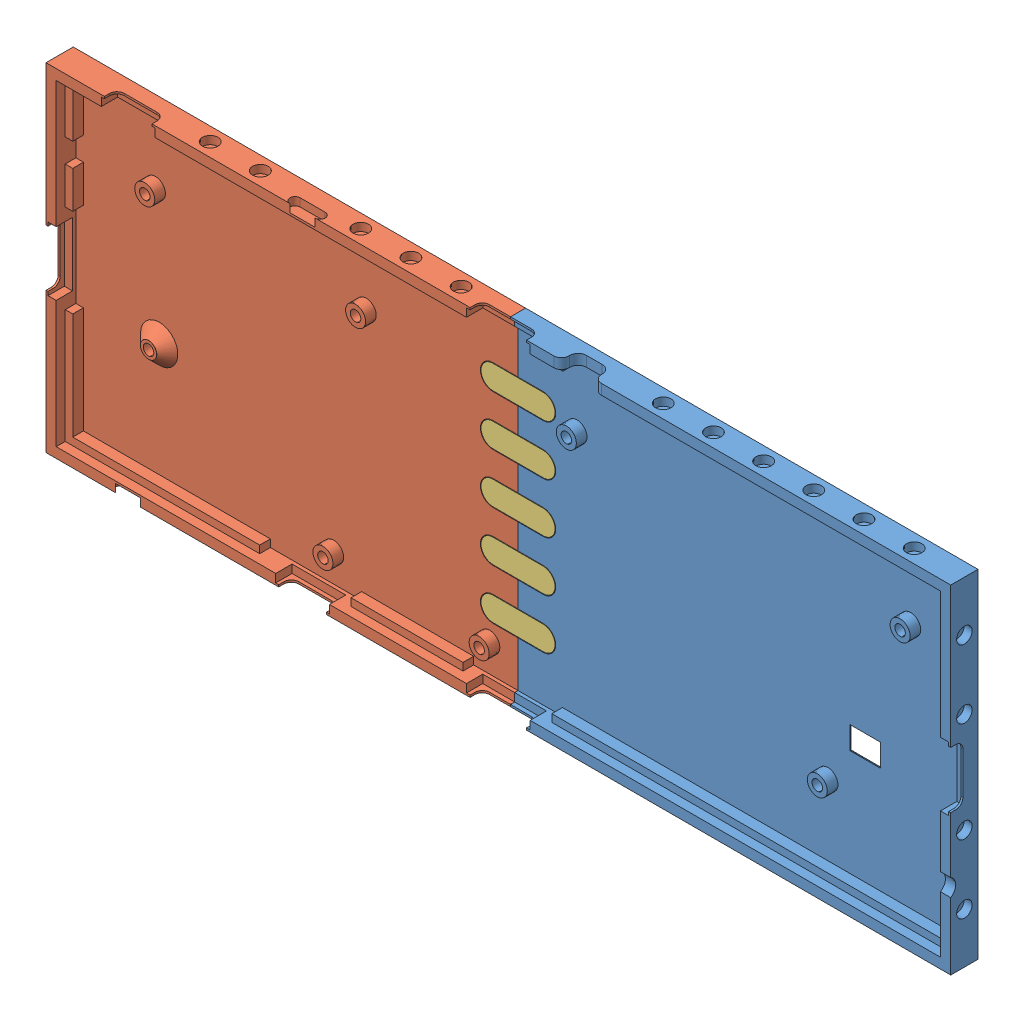
SolidWorks assembly Case, configuration Default. Lengths in mm.
Overall size (360.55 134.6 10.86).
23 component instances, 22 part files, 32 mates.
Components (placement in the parent):
- The Typeuwu.step-1: The Typeuwu.step [Default] at (160.1665 179.2202 272.1358) size (360.55 134.6 14.66) (hidden)
  - The Typeuwu1.step-1: The Typeuwu1.step [Default] at origin size (352.01 126.01 14.66)
  - The Typeuwu2.step-1: The Typeuwu2.step [Default] at origin size (2.96 4.45 1.67)
  - The Typeuwu3.step-1: The Typeuwu3.step [Default] at origin size (0.75 1.95 0)
  - The Typeuwu4.step-1: The Typeuwu4.step [Default] at origin size (0.75 1.95 0)
  - The Typeuwu5.step-1: The Typeuwu5.step [Default] at origin size (2.96 4.45 1.67)
  - The Typeuwu6.step-1: The Typeuwu6.step [Default] at origin size (0.75 1.95 0)
  - The Typeuwu7.step-1: The Typeuwu7.step [Default] at origin size (0.75 1.95 0)
  - The Typeuwu8.step-1: The Typeuwu8.step [Default] at origin size (5 6.4 1.13)
  - The Typeuwu9.step-1: The Typeuwu9.step [Default] at origin size (21 5 8)
  - The Typeuwu10.step-1: The Typeuwu10.step [Default] at origin size (25 5 8)
  - The Typeuwu11.step-1: The Typeuwu11.step [Default] at origin size (21 5 8)
  - The Typeuwu12.step-1: The Typeuwu12.step [Default] at origin size (5 25 8)
  - The Typeuwu13.step-1: The Typeuwu13.step [Default] at origin size (25 5 8)
  - The Typeuwu14.step-1: The Typeuwu14.step [Default] at origin size (5 25 8)
- Base 1-1: Base 1 [Default] at (160.1665 179.2202 270.5242) x (-1 0 0) z (0 0 -1) size (180.3 134.6 10.86)
- Part2-1: Part2 [Default] at (160.1665 179.2202 270.5242) x (-1 0 0) z (0 0 -1) size (180.25 134.56 10.86)
- Buffer 1-1: Buffer 1 [Default] at (160.1665 179.2202 268.5242) size (168.75 126 2) (hidden)
- Buffer 2-1: Buffer 2 [Default] at (160.1665 179.2202 268.5242) size (163.3 126 2) (hidden)
- Plate 1-1: Plate 1 [Default] at (160.1665 179.2202 272.1358) size (198 134.6 4.8) (hidden)
- Buffer Plate 1-1: Buffer Plate 1 [Default] at (160.1665 179.2202 272.1358) size (175.35 97.6 2) (hidden)
- Plate 2-1: Plate 2 [Default] at (160.1665 179.2202 272.1358) size (187.75 134.51 4.8) (hidden)
- Base Binder-1: Base Binder [Default] at (160.1665 179.2202 262.2742) size (29.5 89.5 2)
Mates (geometry in assembly coordinates):
- InPlace1: in place: plane of ? through (160.0633 179.244 270.5242) normal (0 0 -1); plane of ? through (0 0 270.5242) normal (0 0 -1); moOrthogonalPlaneRef_w of ? through (160.0633 179.244 270.5242) normal (0 0 -1); plane of ? through (0 0 270.5242) normal (0 1 0); plane of ? through (160.0633 179.244 270.5242) normal (0 0 -1); plane of ? through (0 0 270.5242) normal (-1 0 0); plane of ? through (160.0633 179.244 270.5242) normal (0 0 -1); unknown of ?
- Coincident1: coincident aligned: plane of ?; plane of ?
- Coincident2: coincident aligned: moOrthogonalPlaneRef_w of The Typeuwu.step-1/The Typeuwu1.step-1 through (160.1665 179.2202 270.5242) normal (0 1 0); plane of Base 1-1 through (160.1665 179.2202 270.5242) normal (0 1 0)
- Coincident3: coincident anti-aligned: moOrthogonalPlaneRef_w of The Typeuwu.step-1/The Typeuwu1.step-1 through (160.1665 179.2202 270.5242) normal (1 0 0); plane of Base 1-1 through (160.1665 179.2202 270.5242) normal (-1 0 0)
- InPlace2: in place: plane of ? through (160.0633 179.244 270.5242) normal (0 0 -1); plane of ? through (0 0 270.5242) normal (0 0 -1); plane of ? through (160.0633 179.244 270.5242) normal (0 0 -1); plane of ? through (0 0 270.5242) normal (0 1 0); plane of ? through (160.0633 179.244 270.5242) normal (0 0 -1); plane of ? through (0 0 270.5242) normal (-1 0 0); plane of ? through (160.0633 179.244 270.5242) normal (0 0 -1); unknown of ?
- Coincident4: coincident aligned: plane of ?; plane of ?
- Coincident5: coincident aligned: moOrthogonalPlaneRef_w of The Typeuwu.step-1/The Typeuwu1.step-1 through (160.1665 179.2202 270.5242) normal (0 1 0); plane of Part2-1 through (160.1665 179.2202 270.5242) normal (0 1 0)
- Coincident6: coincident anti-aligned: moOrthogonalPlaneRef_w of The Typeuwu.step-1/The Typeuwu1.step-1 through (160.1665 179.2202 270.5242) normal (1 0 0); plane of Part2-1 through (160.1665 179.2202 270.5242) normal (-1 0 0)
- InPlace3: in place: plane of ? through (160.0633 179.244 268.5242) normal (0 0 1); plane of ? through (0 0 268.5242) normal (0 0 1); plane of ? through (160.0633 179.244 268.5242) normal (0 0 1); plane of ? through (0 0 268.5242) normal (0 1 0); plane of ? through (160.0633 179.244 268.5242) normal (0 0 1); plane of ? through (0 0 268.5242) normal (1 0 0); plane of ? through (160.0633 179.244 268.5242) normal (0 0 1); unknown of ?
- Coincident1: coincident aligned: plane of ?; plane of ?
- Coincident2: coincident aligned: moOrthogonalPlaneRef_w of Part2-1 through (160.1665 179.2202 268.5242) normal (0 1 0); plane of Buffer 1^Case-1 through (160.1665 179.2202 268.5242) normal (0 1 0)
- Coincident3: coincident anti-aligned: moOrthogonalPlaneRef_w of Part2-1 through (160.1665 179.2202 268.5242) normal (-1 0 0); plane of Buffer 1^Case-1 through (160.1665 179.2202 268.5242) normal (1 0 0)
- InPlace5: in place: plane of ? through (160.0633 179.244 268.5242) normal (0 0 1); plane of ? through (0 0 268.5242) normal (0 0 1); plane of ? through (160.0633 179.244 268.5242) normal (0 0 1); plane of ? through (0 0 268.5242) normal (0 1 0); plane of ? through (160.0633 179.244 268.5242) normal (0 0 1); plane of ? through (0 0 268.5242) normal (1 0 0); plane of ? through (160.0633 179.244 268.5242) normal (0 0 1); unknown of ?
- Coincident7: coincident aligned: plane of ?; plane of ?
- Coincident8: coincident aligned: moOrthogonalPlaneRef_w of Base 1-1 through (160.1665 179.2202 268.5242) normal (0 1 0); plane of Part3^Case-1 through (160.1665 179.2202 268.5242) normal (0 1 0)
- Coincident9: coincident anti-aligned: moOrthogonalPlaneRef_w of Base 1-1 through (160.1665 179.2202 268.5242) normal (-1 0 0); plane of Part3^Case-1 through (160.1665 179.2202 268.5242) normal (1 0 0)
- InPlace6: in place: plane of ? through (160.1665 421.1551 272.1358) normal (0 0 1); plane of ? through (0 0 272.1358) normal (0 0 1); plane of ? through (160.1665 421.1551 272.1358) normal (0 0 1); plane of ? through (0 0 272.1358) normal (0 1 0); plane of ? through (160.1665 421.1551 272.1358) normal (0 0 1); plane of ? through (0 0 272.1358) normal (1 0 0); plane of ? through (160.1665 421.1551 272.1358) normal (0 0 1); unknown of ?
- Coincident1: coincident aligned: plane of ?; plane of ?
- Coincident2: coincident aligned: moOrthogonalPlaneRef_w of Part2-1 through (160.1665 179.2202 272.1358) normal (0 1 0); plane of Plate 1-1 through (160.1665 179.2202 272.1358) normal (0 1 0)
- Coincident3: coincident anti-aligned: moOrthogonalPlaneRef_w of Part2-1 through (160.1665 179.2202 272.1358) normal (-1 0 0); plane of Plate 1-1 through (160.1665 179.2202 272.1358) normal (1 0 0)
- InPlace7: in place: plane of ? through (160.0633 179.244 272.1358) normal (0 0 1); plane of ? through (0 0 272.1358) normal (0 0 1); plane of ? through (160.0633 179.244 272.1358) normal (0 0 1); plane of ? through (0 0 272.1358) normal (0 1 0); plane of ? through (160.0633 179.244 272.1358) normal (0 0 1); plane of ? through (0 0 272.1358) normal (1 0 0); plane of ? through (160.0633 179.244 272.1358) normal (0 0 1); unknown of ?
- Coincident4: coincident aligned: plane of ?; plane of ?
- Coincident5: coincident aligned: moOrthogonalPlaneRef_w of The Typeuwu.step-1/The Typeuwu1.step-1 through (160.1665 179.2202 272.1358) normal (0 1 0); plane of Buffer Plate 1-1 through (160.1665 179.2202 272.1358) normal (0 1 0)
- Coincident6: coincident anti-aligned: moOrthogonalPlaneRef_w of The Typeuwu.step-1/The Typeuwu1.step-1 through (160.1665 179.2202 272.1358) normal (-1 0 0); plane of Buffer Plate 1-1 through (160.1665 179.2202 272.1358) normal (1 0 0)
- InPlace8: in place: plane of ? through (160.0633 179.244 272.1358) normal (0 0 1); plane of ? through (0 0 272.1358) normal (0 0 1); plane of ? through (160.0633 179.244 272.1358) normal (0 0 1); plane of ? through (0 0 272.1358) normal (0 1 0); plane of ? through (160.0633 179.244 272.1358) normal (0 0 1); plane of ? through (0 0 272.1358) normal (1 0 0); plane of ? through (160.0633 179.244 272.1358) normal (0 0 1); unknown of ?
- Coincident7: coincident aligned: plane of ?; plane of ?
- Coincident8: coincident aligned: moOrthogonalPlaneRef_w of The Typeuwu.step-1/The Typeuwu1.step-1 through (160.1665 179.2202 272.1358) normal (0 1 0); plane of Plate 2-1 through (160.1665 179.2202 272.1358) normal (0 1 0)
- Coincident9: coincident anti-aligned: moOrthogonalPlaneRef_w of The Typeuwu.step-1/The Typeuwu1.step-1 through (160.1665 179.2202 272.1358) normal (-1 0 0); plane of Plate 2-1 through (160.1665 179.2202 272.1358) normal (1 0 0)
- InPlace9: in place: plane of ? through (170.1665 179.2202 262.2742) normal (0 0 1); plane of ? through (0 0 262.2742) normal (0 0 1); plane of ? through (170.1665 179.2202 262.2742) normal (0 0 1); plane of ? through (0 0 262.2742) normal (0 1 0); plane of ? through (170.1665 179.2202 262.2742) normal (0 0 1); plane of ? through (0 0 262.2742) normal (1 0 0); plane of ? through (170.1665 179.2202 262.2742) normal (0 0 1); unknown of Base Binder-1
- Coincident1: coincident aligned: plane of ?; plane of ?
- Coincident2: coincident aligned: moOrthogonalPlaneRef_w of Part2-1 through (160.1665 179.2202 262.2742) normal (0 1 0); plane of Part1^Case-1 through (160.1665 179.2202 262.2742) normal (0 1 0)
- Coincident3: coincident anti-aligned: moOrthogonalPlaneRef_w of Part2-1 through (160.1665 179.2202 262.2742) normal (-1 0 0); plane of Part1^Case-1 through (160.1665 179.2202 262.2742) normal (1 0 0)
